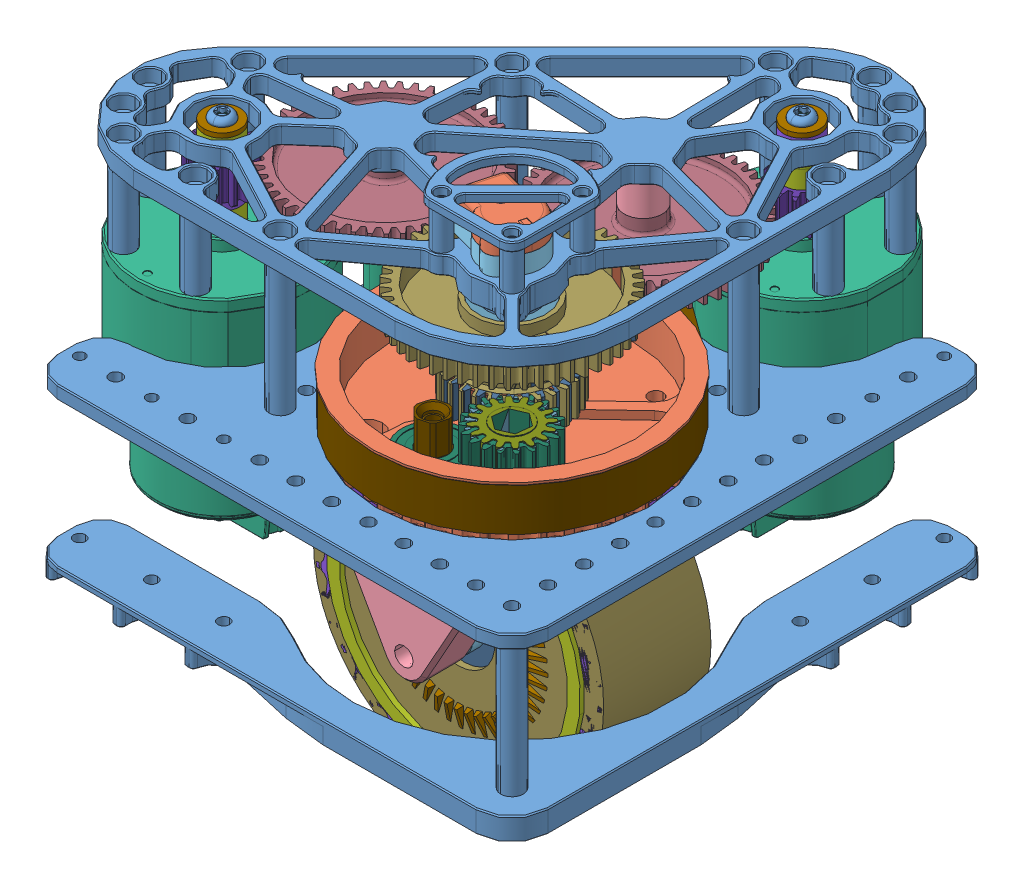
SolidWorks assembly SimMK4BL, configuration Default. Lengths in mm.
Overall size (204.6 195.06 203.54).
60 component instances, 41 part files, 5 mates.
Components (placement in the parent):
- MK4Frame-1: MK4Frame [Default] at origin size (189.87 134.14 189.87)
  - MK4i Master Part_Default Falcon 500 Config.STEP-1: MK4i Master Part_Default Falcon 500 Config.STEP [Default] at origin size (189.87 134.14 189.87)
  - Bearing, R188ZZ, 217-3489.STEP-1: Bearing, R188ZZ, 217-3489.STEP [Default] at (-77.6314 97.6313 -123.9376) x (-0.188457 0 -0.982081) z (0.982081 0 -0.188457) size (12.7 4.76 12.7)
  - Bearing, 688.STEP-1: Bearing, 688.STEP [Default] at (-77.6314 150.1375 -123.9376) x (0 -1 0) z (-0.336154 0 0.941807) size (5 16 16)
  - MK4i Steering Shaft Spacer.STEP-1: MK4i Steering Shaft Spacer.STEP [Default] at (-77.6314 134.8105 -123.9376) x (-0.728275 0 -0.685285) z (0.685285 0 -0.728275) size (13.36 12.7 13.36)
  - MK4i Steering Shaft Tall.STEP-1: MK4i Steering Shaft Tall.STEP [Default] at (-77.6314 152.5105 -123.9376) x (0.998641 0 -0.05212) z (0.05212 0 0.998641) size (17.78 57.04 17.78)
  - MK4i Shaft, Drive Idler.STEP-1: MK4i Shaft, Drive Idler.STEP [Default] at (-128.0498 100.0125 -83.2602) size (13.36 56.18 13.36)
  - Falcon Spacer .25.STEP-1: Falcon Spacer .25.STEP [Default] at (-158.75 123.7 -56.515) x (0.995401 0 0.095792) z (-0.095792 0 0.995401) size (12.7 6.35 12.7)
  - Falcon Spacer .25.STEP-2: Falcon Spacer .25.STEP [Default] at (-158.75 145.925 -56.515) x (0.92897 0 -0.370156) z (0.370156 0 0.92897) size (12.7 6.35 12.7)
  - Falcon Spacer .125.STEP-1: Falcon Spacer .125.STEP [Default] at (-56.515 149.1 -158.75) x (0.944247 0 -0.329237) z (0.329237 0 0.944247) size (12.7 3.17 12.7)
  - Falcon Spacer .125.STEP-2: Falcon Spacer .125.STEP [Default] at (-158.75 130.05 -56.515) x (0.865282 0 -0.501286) z (0.501286 0 0.865282) size (12.7 3.17 12.7)
  - Falcon Spacer .0625.STEP-1: Falcon Spacer .0625.STEP [Default] at (-158.75 152.275 -56.515) size (12.7 1.59 12.7)
  - Falcon Spacer .0625.STEP-2: Falcon Spacer .0625.STEP [Default] at (-56.515 152.275 -158.75) x (0.982082 0 -0.188455) z (0.188455 0 0.982082) size (12.7 1.59 12.7)
  - Falcon Spacer .25.STEP-3: Falcon Spacer .25.STEP [Default] at (-56.515 136.4 -158.75) size (12.7 6.35 12.7)
  - Falcon Spacer .25.STEP-4: Falcon Spacer .25.STEP [Default] at (-56.515 142.75 -158.75) x (0.982082 0 -0.188455) z (0.188455 0 0.982082) size (12.7 6.35 12.7)
  - Copy of topgears-1: Copy of topgears [Default] at origin size (163.42 43.94 160.87)
    - Double Gear, 20DP, 27T, 50T.STEP-1: Double Gear, 20DP, 27T, 50T.STEP [Default] at (-66.675 110.1225 -66.675) x (-0.730582 0 -0.682825) z (0 1 0) size (65.97 66.04 34.49)
    - Double Gear, 20DP, 25T, 50T.STEP-1: Double Gear, 20DP, 25T, 50T.STEP [Default] at (-66.675 110.1225 -66.675) x (-0.730582 0 -0.682825) z (0 1 0) size (65.97 66.04 34.49)
    - Double Gear, 20DP, 28T, 50T.STEP-1: Double Gear, 20DP, 28T, 50T.STEP [Default] at (-66.675 110.1225 -66.675) x (-0.730582 0 -0.682825) z (0 1 0) size (65.97 66.04 34.49)
    - Gear, 50T, 20DP, .375Hex.STEP-1: Gear, 50T, 20DP, .375Hex.STEP [Default] at (-128.0498 139.8651 -83.2602) x (0.985885 0 -0.167422) z (0 1 0) size (65.97 66.04 12.65)
    - Gear, 50T, 20DP, .375Hex.STEP-2: Gear, 50T, 20DP, .375Hex.STEP [Default] at (-77.6314 128.4859 -123.9376) x (-0.963721 0 0.266911) z (0 1 0) size (65.97 66.04 12.65)
    - Gear, 17T, 20DP, .375Hex.STEP-1: Gear, 17T, 20DP, .375Hex.STEP [Default] at (-46.8646 115.8367 -46.8646) x (0 1 0) z (0.115868 0 -0.993265) size (12.6 23.99 24.09)
    - Gear, 19T, 20DP, .375Hex.STEP-1: Gear, 19T, 20DP, .375Hex.STEP [Default] at (-46.8646 115.8367 -46.8646) x (0.115868 0 -0.993265) z (0.993265 0 0.115868) size (26.55 12.6 26.64)
    - Gear, 20DP, 16T, .375Hex, 217-5451.STEP-1: Gear, 20DP, 16T, .375Hex, 217-5451.STEP [Default] at (-46.8646 115.8375 -46.8646) x (0.993265 0 0.115868) z (0 -1 0) size (22.6 22.6 12.6)
    - Gear, 20DP 14T, Falcon Spline, am-4147.STEP-1: Gear, 20DP 14T, Falcon Spline, am-4147.STEP [Default] at (-56.515 123.7 -158.75) x (0 1 0) z (-0.155924 0 -0.987769) size (12.71 19.97 20.32)
    - Gear, 20DP 14T, Falcon Spline, am-4147.STEP-2: Gear, 20DP 14T, Falcon Spline, am-4147.STEP [Default] at (-158.75 133.225 -56.515) x (0 1 0) z (-0.622557 0 -0.782574) size (12.71 19.97 20.32)
    - Belt, 320-5M-15.STEP-1: Belt, 320-5M-15.STEP [Default] at (-66.675 109.752 -66.675) x (0.982183 0 -0.187927) z (0.187927 0 0.982183) size (97.78 15 116.29)
  - Bearing, 688.STEP-2: Bearing, 688.STEP [Default] at (-128.0498 97.5125 -83.2602) x (0 -1 0) z (-0.444562 0 0.895748) size (5 16 16)
  - Screw, Falcon 500 Pinion_90939A124.STEP-1: Screw, Falcon 500 Pinion_90939A124.STEP [Default] at (-56.515 153.8625 -158.75) x (1 0 0) z (0 1 0) size (7.93 7.93 14.91)
  - Screw, Falcon 500 Pinion_90939A124.STEP-2: Screw, Falcon 500 Pinion_90939A124.STEP [Default] at (-158.75 153.8625 -56.515) x (0.982082 0 -0.188455) z (0 1 0) size (7.93 7.93 14.91)
  - CANcoder Assembly.STEP-1: CANcoder Assembly.STEP [Default] at (-66.675 132.3975 -66.675) x (-0.260871 0 0.965374) z (0 1 0) size (21.75 26.91 13.52)
    - CANcoder Top Housing.STEP-1: CANcoder Top Housing.STEP [Default] at origin size (21.53 26.79 8.94)
    - CANcoder PCA.STEP-1: CANcoder PCA.STEP [Default] at (0 0 22.3055) size (15.93 23.27 3.19)
    - CANcoder Screw.STEP-1: CANcoder Screw.STEP [Default] at origin size (4.24 4.24 12.65)
    - CANcoder Bottom Housing.STEP-1: CANcoder Bottom Housing.STEP [Default] at origin size (21.75 26.91 6.35)
- MK4Motors-1: MK4Motors [Default] at (0 0.6375 0) size (162.75 116.08 164.3)
  - Motor, Falcon500.STEP-1: Motor, Falcon500.STEP [Default] at (-158.75 82.1244 -56.515) x (0 0 1) z (0 1 0) size (61.56 60.51 116.08)
  - Motor, Falcon500.STEP-2: Motor, Falcon500.STEP [Default] at (-56.515 82.1244 -158.75) x (-1 0 0) z (0 1 0) size (61.56 60.51 116.08)
- MK4wheel-1: MK4wheel [Default] at (-21.7078 74.7442 27.2182) x (-0.340538 0.616743 0.709692) z (0.35119 -0.616743 0.704482) size (128.67 139.68 128.67)
  - MK4 Billet Wheel Assembly.STEP-1: MK4 Billet Wheel Assembly.STEP [Default] at (-66.675 50.7435 -66.675) x (0.707107 0 0.707107) z (0.41117 0.813559 -0.41117) size (42.28 100.13 100.13)
    - Wheel, SDS, Nitrile Tread, 4in X 1.5in, Bearing Bore.STEP-1: Wheel, SDS, Nitrile Tread, 4in X 1.5in, Bearing Bore.STEP [Default] at origin size (42.28 88.9 88.9)
    - Tread, Blue Nitrile 4in X 1.5in.STEP-1: Tread, Blue Nitrile 4in X 1.5in.STEP [Default] at origin size (38.1 100.13 100.13)
  - Bevel Gear, 4515.STEP-1: Bevel Gear, 4515.STEP [Default] at (-54.7746 50.7435 -54.7746) x (0.575273 -0.581482 -0.575273) z (-0.41117 -0.813559 0.41117) size (68.38 7.77 68.42)
  - Bearing, R8ZZ.STEP-1: Bearing, R8ZZ.STEP [Default] at (-57.5286 50.7435 -57.5286) x (-0.158587 -0.974526 0.158587) z (-0.689094 0.224275 0.689094) size (28.57 7.94 28.57)
  - Bearing, R6ZZ.STEP-1: Bearing, R6ZZ.STEP [Default] at (-79.2721 50.7435 -79.2721) x (-0.694824 0.18558 0.694824) z (0.131225 0.982629 -0.131225) size (22.23 7.14 22.23)
  - WheelCollision-1: WheelCollision [Rev 1.1] at (-80.1454 50.7435 -80.1454) x (0.706764 -0.031147 -0.706764) z (0.707107 0 0.707107) size (101.6 101.6 38.1)
- MK4WheelMount-1: MK4WheelMount [Default] at (-65.9648 -0.82 27.615) x (0.712413 0 0.701761) z (-0.701761 0 0.712413) size (139.19 113.33 139.19)
  - Shim, 8mm ID X 14mm OD X .5mm Thick, 98055A115_98055A115.STEP-1: Shim, 8mm ID X 14mm OD X .5mm Thick, 98055A115_98055A115.STEP [Default] at (-46.8646 73.9775 -46.8646) x (0.942304 0 -0.334759) z (0.334759 0 0.942304) size (14 1 14)
  - Bearing, 6802.STEP-1: Bearing, 6802.STEP [Default] at (-66.675 138.5216 -66.675) x (0.972423 0 0.233226) z (-0.233226 0 0.972423) size (24 5 24)
  - Bearing, 6802.STEP-2: Bearing, 6802.STEP [Default] at (-66.675 118.1216 -66.675) x (0.639486 0 0.768802) z (-0.768802 0 0.639486) size (24 5 24)
  - Bearing, 688.STEP-1: Bearing, 688.STEP [Default] at (-46.8646 71.4775 -46.8646) x (0 -1 0) z (-0.336154 0 0.941807) size (5 16 16)
  - Bearing, .375 ThunderHex, Flanged, 217-5829.STEP-1: Bearing, .375 ThunderHex, Flanged, 217-5829.STEP [Default] at (-46.8646 102.3938 -46.8646) x (0.903016 0 0.429606) z (-0.429606 0 0.903016) size (24.51 7.14 24.51)
  - Bevel Gear, 1545.STEP-1: Bevel Gear, 1545.STEP [Default] at (-46.8646 84.4935 -46.8646) x (-0.830686 0 -0.556741) z (-0.556741 0 0.830686) size (28.28 15.37 25.62)
  - Bearing, A035XPO_SA035XPO.STEP-1: Bearing, A035XPO_SA035XPO.STEP [Default] at (-66.675 95.25 -66.675) x (0.978935 0 0.20417) z (-0.20417 0 0.978935) size (101.6 6.35 101.6)
  - MK4 Intermediate Shaft.STEP-1: MK4 Intermediate Shaft.STEP [Default] at (-46.8646 68.3577 -46.8646) x (0.999953 0 0.009669) z (-0.009669 0 0.999953) size (11.68 51.44 11.68)
  - MK3 Center Column.STEP-1: MK3 Center Column.STEP [Default] at (-66.675 113.0816 -66.675) x (-0.707107 0 0.707107) z (-0.707107 0 -0.707107) size (17.27 40.32 17.27)
  - MK3 Base Pulley Tall.STEP-1: MK3 Base Pulley Tall.STEP [Default] at (-66.675 98.425 -66.675) x (-0.707107 0 0.707107) z (-0.707107 0 -0.707107) size (98.42 27.08 98.42)
  - Wheel Mount A.STEP-1: Wheel Mount A.STEP [Default] at (-88.2276 50.7435 -88.2276) x (-0.707107 0 -0.707107) z (0.707107 0 -0.707107) size (17.09 49.74 57.15)
  - Wheel Mount B Gen2.STEP-1: Wheel Mount B Gen2.STEP [Default] at (-45.1224 50.7435 -45.1224) x (-0.707107 0 -0.707107) z (0.707107 0 -0.707107) size (15.88 49.27 57.15)
  - MK4 Wheel Spacer.STEP-1: MK4 Wheel Spacer.STEP [Default] at (-76.7015 50.7435 -76.7015) x (-0.707107 0 -0.707107) z (0.522819 -0.67329 -0.522819) size (36.72 15.11 15.11)
Mates (geometry in assembly coordinates):
- Concentric1: concentric anti-aligned: cylinder of MK4Frame-1/Falcon Spacer .25.STEP-1 through (-158.75 130.05 -56.515) axis (0 -1 0) radius 3.75; cylinder of MK4Motors-1/Motor, Falcon500.STEP-1 through (-158.75 154.5 -56.515) axis (0 1 0) radius 1.7272
- Coincident1: coincident anti-aligned: plane of MK4Frame-1/Falcon Spacer .25.STEP-1 through (-158.75 123.7 -56.515) normal (0 -1 0); plane of MK4Motors-1/Motor, Falcon500.STEP-1 through (-158.75 123.7 -62.515) normal (0 1 0)
- Coincident2: coincident anti-aligned: circle of MK4Frame-1/Copy of topgears-1/Belt, 320-5M-15.STEP-1; cone of MK4WheelMount-1/MK3 Base Pulley Tall.STEP-1 through (-66.675 116.813 -66.675) axis (0 -1 0)
- Coincident3: coincident anti-aligned: plane of MK4wheel-1/Bearing, R8ZZ.STEP-1 through (-66.5482 49.9235 -49.8353) normal (0.007532 0 0.999972); plane of MK4WheelMount-1/MK4 Wheel Spacer.STEP-1 through (-61.4606 55.5106 -49.8736) normal (-0.007532 0 -0.999972)
- Concentric4: concentric anti-aligned: cylinder of MK4wheel-1/Bearing, R8ZZ.STEP-1 through (-66.5482 49.9235 -49.8353) axis (-0.007532 0 -0.999972) radius 6.35; cylinder of MK4WheelMount-1/Wheel Mount B Gen2.STEP-1 through (-66.3856 49.9235 -28.2586) axis (0.007532 0 0.999972) radius 3.2639
